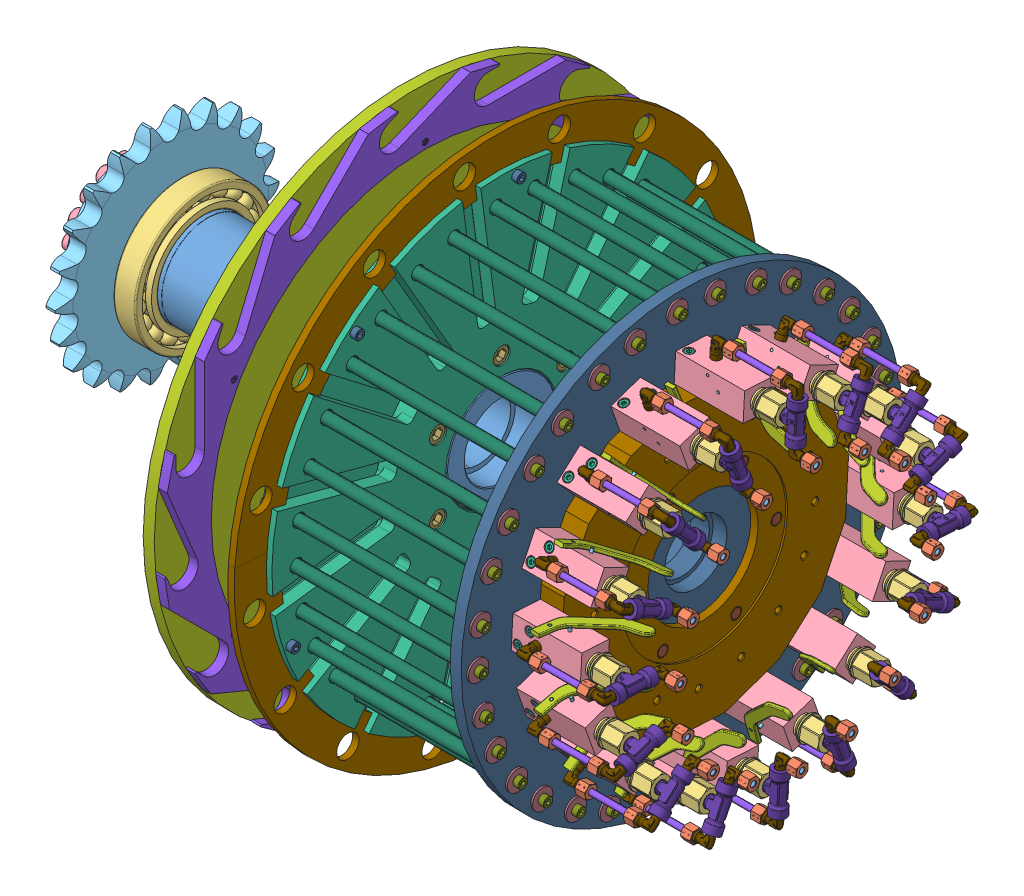
SolidWorks assembly assieme parte rotante, configuration Default. Lengths in mm.
Overall size (749.63 778.63 778.63).
555 component instances, 28 part files, 75 mates.
Components (placement in the parent):
- albero rotazione piatti-1: albero rotazione piatti [Default] at (60.413 18.3637 415) size (415 200 200)
- seger 100mm-1: seger 100mm [KS 1336 E - 100] at (-146.4567 18.3637 415) x (0 0 -1) z (1 0 0) size (107.55 112.98 3)
- SKF - 6020 - 20,DE,NC,20_68-1: SKF - 6020 - 20,DE,NC,20_68 [SKF - 6020 - 20,DE,NC,20_68] at (-131.4567 18.3637 415) x (1 0 0) z (0 -0.434476 -0.900684) size (24 150 150)
- calettatore d95-1: calettatore d95 [Default] at (-184.9572 18.3637 415) size (39.5 135 135)
- pulegia z =50-1: pulegia z =50 [Chain wheel ISO - 22Z 20A-1 --22SB150H40L95.0N] at (-173.9167 18.3637 415) size (40 241.57 243.73)
- Disco supporto montaggio e Colonne-1: Disco supporto montaggio e Colonne [Default] at (204.0433 18.3637 415) x (0 -0.866025 -0.5) z (1 0 0) size (499.6 499.6 29)
- SKF - 6020 - 20,DE,NC,20_68-2: SKF - 6020 - 20,DE,NC,20_68 [SKF - 6020 - 20,DE,NC,20_68] at (62.0433 18.3637 415) x (1 0 0) z (0 -0.432628 -0.901573) size (24 150 150)
- piatto rotante porta tappi-1: piatto rotante porta tappi [Default] at (99.0433 18.3637 415) x (0 0 -1) z (1 0 0) size (570 570 20.57)
- disco trasportatore tappi 31-1: disco trasportatore tappi 31 [Default] at (111.0433 18.3637 415) x (0 0.5 -0.866025) z (1 0 0) size (570 570 10.42)
- Distributore Rotante-1: Distributore Rotante [Default] at (425.0433 18.3637 415) x (0 -0.055301 -0.99847) z (1 0 0) size (310 310 25.54)
- disco trascinato porta distributore vuoto-1: disco trascinato porta distributore vuoto [Default] at (400.0433 18.3637 415) x (0 0.055301 0.99847) z (-1 0 0) size (480 480 50)
- m12 35mm-1: m12 35mm [ISO 4762 M12 x 35 - 35N] at (376.0433 -53.0243 378.8925) x (1 0 0) z (0 -0.5 0.866025) size (47 18 18)
- m12 90mm-3: m12 90mm [ISO 4762 M12 x 90 - 90N] at (203.0433 -21.6363 345.718) x (-1 0 0) z (0 -0.5 0.866025) size (102 18 18)
- rondella m6 22mm-1: rondella m6 22mm [Washer ISO 7094 - 6] at (99.0433 -101.6363 207.1539) x (1 0 0) z (0 -1 0) size (2 22 22)
- M6 20mm-1: M6 20mm [ISO 4762 M6 x 20 - 20N] at (91.0433 -101.6363 207.1539) x (1 0 0) z (0 0.5 0.866025) size (26 10 10)
- m12 35mm-2: m12 35mm [ISO 4762 M12 x 35 - 35N] at (376.0433 13.9397 335.1224) x (1 0 0) z (0 -1 0) size (47 18 18)
- m12 35mm-3: m12 35mm [ISO 4762 M12 x 35 - 35N] at (376.0433 85.3277 371.2299) x (1 0 0) z (0 -0.5 -0.866025) size (47 18 18)
- m12 35mm-4: m12 35mm [ISO 4762 M12 x 35 - 35N] at (376.0433 89.7517 451.1075) x (1 0 0) z (0 0.5 -0.866025) size (47 18 18)
- m12 35mm-5: m12 35mm [ISO 4762 M12 x 35 - 35N] at (376.0433 22.7877 494.8776) x (1 0 0) z (0 1 0) size (47 18 18)
- m12 35mm-6: m12 35mm [ISO 4762 M12 x 35 - 35N] at (376.0433 -48.6003 458.7701) x (1 0 0) z (0 0.5 0.866025) size (47 18 18)
- rondella m6 22mm-2: rondella m6 22mm [Washer ISO 7094 - 6] at (99.0433 138.3637 207.1539) x (1 0 0) z (0 -0.5 -0.866025) size (2 22 22)
- rondella m6 22mm-3: rondella m6 22mm [Washer ISO 7094 - 6] at (99.0433 258.3637 415) x (1 0 0) z (0 0.5 -0.866025) size (2 22 22)
- rondella m6 22mm-4: rondella m6 22mm [Washer ISO 7094 - 6] at (99.0433 138.3637 622.8461) x (1 0 0) z (0 1 0) size (2 22 22)
- rondella m6 22mm-5: rondella m6 22mm [Washer ISO 7094 - 6] at (99.0433 -101.6363 622.8461) x (1 0 0) z (0 0.5 0.866025) size (2 22 22)
- rondella m6 22mm-6: rondella m6 22mm [Washer ISO 7094 - 6] at (99.0433 -221.6363 415) x (1 0 0) z (0 -0.5 0.866025) size (2 22 22)
- M6 20mm-2: M6 20mm [ISO 4762 M6 x 20 - 20N] at (91.0433 138.3637 207.1539) x (1 0 0) z (0 -0.5 0.866025) size (26 10 10)
- M6 20mm-3: M6 20mm [ISO 4762 M6 x 20 - 20N] at (91.0433 258.3637 415) x (1 0 0) z (0 -1 0) size (26 10 10)
- M6 20mm-4: M6 20mm [ISO 4762 M6 x 20 - 20N] at (91.0433 138.3637 622.8461) x (1 0 0) z (0 -0.5 -0.866025) size (26 10 10)
- M6 20mm-5: M6 20mm [ISO 4762 M6 x 20 - 20N] at (91.0433 -101.6363 622.8461) x (1 0 0) z (0 0.5 -0.866025) size (26 10 10)
- M6 20mm-6: M6 20mm [ISO 4762 M6 x 20 - 20N] at (91.0433 -221.6363 415) x (1 0 0) z (0 1 0) size (26 10 10)
- m12 90mm-4: m12 90mm [ISO 4762 M12 x 90 - 90N] at (203.0433 58.3637 345.718) x (-1 0 0) z (0 -1 0) size (102 18 18)
- m12 90mm-5: m12 90mm [ISO 4762 M12 x 90 - 90N] at (203.0433 98.3637 415) x (-1 0 0) z (0 -0.5 -0.866025) size (102 18 18)
- m12 90mm-6: m12 90mm [ISO 4762 M12 x 90 - 90N] at (203.0433 58.3637 484.282) x (-1 0 0) z (0 0.5 -0.866025) size (102 18 18)
- m12 90mm-7: m12 90mm [ISO 4762 M12 x 90 - 90N] at (203.0433 -21.6363 484.282) x (-1 0 0) z (0 1 0) size (102 18 18)
- m12 90mm-8: m12 90mm [ISO 4762 M12 x 90 - 90N] at (203.0433 -61.6363 415) x (-1 0 0) z (0 0.5 0.866025) size (102 18 18)
- asta scorrimento carello-1: asta scorrimento carello [Default] at (287.5433 70.1437 197.9013) x (0 0 -1) z (1 0 0) size (12 12 225)
- rondella m6 22mm-7: rondella m6 22mm [Washer ISO 7094 - 6] at (175.0433 70.1437 197.9013) x (1 0 0) z (0 -1 0) size (2 22 22)
- M6 16mm-1: M6 16mm [ISO 4762 M6 x 16 - 16N] at (167.0433 70.1437 197.9013) size (22 10 10)
- M6 16mm-2: M6 16mm [ISO 4762 M6 x 16 - 16N] at (408.0433 70.1437 197.9013) x (-1 0 0) z (0 0 -1) size (22 10 10)
- rondella m6 22mm-8: rondella m6 22mm [Washer ISO 7094 - 6] at (400.0433 70.1437 197.9013) x (-1 0 0) z (0 1 0) size (2 22 22)
- rondella m6 22mm-9: rondella m6 22mm [Washer ISO 7094 - 6] at (175.0433 24.5373 191.8971) x (1 0 0) z (0 -0.965926 -0.258819) size (2 22 22)
- M6 16mm-3: M6 16mm [ISO 4762 M6 x 16 - 16N] at (167.0433 24.5373 191.8971) x (1 0 0) z (0 0.258819 -0.965926) size (22 10 10)
- asta scorrimento carello-2: asta scorrimento carello [Default] at (287.5433 24.5373 191.8971) x (0 0.258819 -0.965926) z (-1 0 0) size (12 12 225)
- rondella m6 22mm-10: rondella m6 22mm [Washer ISO 7094 - 6] at (400.0433 24.5373 191.8971) x (-1 0 0) z (0 0.965926 0.258819) size (2 22 22)
- M6 16mm-4: M6 16mm [ISO 4762 M6 x 16 - 16N] at (408.0433 24.5373 191.8971) x (-1 0 0) z (0 -0.258819 0.965926) size (22 10 10)
- AssiemeValvola-1: AssiemeValvola [Default] at (515.3257 74.6348 254.5832) x (0 -0.331007 0.943628) z (0 0.943628 0.331007) size (90.26 138.63 38)
  - RaccordoT-1: RaccordoT [Default] at origin size (43 29.75 16.5)
  - Raccordo a L-1: Raccordo a L [Default] at (-30 0 0) x (0 -1 0) z (0 0 -1) size (28.34 25.51 14.01)
    - 1809_06_10_01-1: 1809_06_10_01 [Default] at origin size (22.49 23 10)
    - 1809_06_10_02-1: 1809_06_10_02 [Default] at origin size (6.5 8.5 8.5)
    - 1809_06_10_03-1: 1809_06_10_03 [Default] at origin size (11.02 15.01 14.01)
  - Raccordo a L-2: Raccordo a L [Default] at (30 0 0) x (0 1 0) z (0 0 -1) size (28.34 25.51 14.01)
    - 1809_06_10_01-1: 1809_06_10_01 [Default] at origin size (22.49 23 10)
    - 1809_06_10_02-1: 1809_06_10_02 [Default] at origin size (6.5 8.5 8.5)
    - 1809_06_10_03-1: 1809_06_10_03 [Default] at origin size (11.02 15.01 14.01)
  - TappoChiusura-1: TappoChiusura [Default] at (0 -32 0) x (0 -1 0) z (0 0 1) size (38.28 26.74 26.74)
  - CorpoValvola-1: CorpoValvola [Default] at (-15 -115.2824 0) size (30 75 34)
  - Raccordo a L-3: Raccordo a L [Default] at (-30 -88.2824 0) x (0 1 0) z (0 0 1) size (28.34 25.51 14.01)
    - 1809_06_10_01-1: 1809_06_10_01 [Default] at origin size (22.49 23 10)
    - 1809_06_10_02-1: 1809_06_10_02 [Default] at origin size (6.5 8.5 8.5)
    - 1809_06_10_03-1: 1809_06_10_03 [Default] at origin size (11.02 15.01 14.01)
  - Spina_3x38-1: Spina_3x38 [Default] at (0 -68.2824 -21) x (-1 0 0) z (0 0 1) size (3 3 38)
  - Spina_3x38-2: Spina_3x38 [Default] at (-10 -80.2824 -21) x (0.996193 0.087174 0) z (0 0 1) size (3 3 38)
  - M5 40mm-3: M5 40mm [ISO 4762 M5 x 40 - 40N] at (-14.6 -108.7824 9) size (45 8.5 8.5)
  - M5 40mm-2: M5 40mm [ISO 4762 M5 x 40 - 40N] at (-14.6 -96.7824 -9) size (45 8.5 8.5)
  - LevaValvola-1: LevaValvola [Default] at (-24.507 -86.571 -17) x (0.996193 0.087174 0) z (0 0 1) size (77.55 60.2 4)
  - Tubo-1: Tubo [Default] at (-30 -15.9665 0) x (1 0 0) z (0 -1 0) size (6 6 56.4)
- M6 16mm-5: M6 16mm [ISO 4762 M6 x 16 - 16N] at (167.0433 -16.8778 194.6116) x (1 0 0) z (0 0.382683 0.92388) size (22 10 10)
- M6 16mm-6: M6 16mm [ISO 4762 M6 x 16 - 16N] at (167.0433 -98.5342 224.874) x (1 0 0) z (0 0.707107 0.707107) size (22 10 10)
- M6 16mm-7: M6 16mm [ISO 4762 M6 x 16 - 16N] at (167.0433 -162.3939 284.0814) x (1 0 0) z (0 0.92388 0.382683) size (22 10 10)
- M6 16mm-8: M6 16mm [ISO 4762 M6 x 16 - 16N] at (167.0433 -198.735 363.22) x (1 0 0) z (0 1 0) size (22 10 10)
- M6 16mm-9: M6 16mm [ISO 4762 M6 x 16 - 16N] at (167.0433 -202.0247 450.2415) x (1 0 0) z (0 0.92388 -0.382683) size (22 10 10)
- M6 16mm-10: M6 16mm [ISO 4762 M6 x 16 - 16N] at (167.0433 -171.7623 531.8979) x (1 0 0) z (0 0.707107 -0.707107) size (22 10 10)
- M6 16mm-11: M6 16mm [ISO 4762 M6 x 16 - 16N] at (167.0433 -112.5549 595.7576) x (1 0 0) z (0 0.382683 -0.92388) size (22 10 10)
- M6 16mm-12: M6 16mm [ISO 4762 M6 x 16 - 16N] at (167.0433 -33.4163 632.0987) x (1 0 0) z (0 0 -1) size (22 10 10)
- M6 16mm-13: M6 16mm [ISO 4762 M6 x 16 - 16N] at (167.0433 53.6052 635.3884) x (1 0 0) z (0 -0.382683 -0.92388) size (22 10 10)
- M6 16mm-14: M6 16mm [ISO 4762 M6 x 16 - 16N] at (167.0433 135.2616 605.126) x (1 0 0) z (0 -0.707107 -0.707107) size (22 10 10)
- M6 16mm-15: M6 16mm [ISO 4762 M6 x 16 - 16N] at (167.0433 199.1213 545.9186) x (1 0 0) z (0 -0.92388 -0.382683) size (22 10 10)
- M6 16mm-16: M6 16mm [ISO 4762 M6 x 16 - 16N] at (167.0433 235.4624 466.78) x (1 0 0) z (0 -1 0) size (22 10 10)
- M6 16mm-17: M6 16mm [ISO 4762 M6 x 16 - 16N] at (167.0433 238.7521 379.7585) x (1 0 0) z (0 -0.92388 0.382683) size (22 10 10)
- M6 16mm-18: M6 16mm [ISO 4762 M6 x 16 - 16N] at (167.0433 208.4897 298.1021) x (1 0 0) z (0 -0.707107 0.707107) size (22 10 10)
- M6 16mm-19: M6 16mm [ISO 4762 M6 x 16 - 16N] at (167.0433 149.2823 234.2424) x (1 0 0) z (0 -0.382683 0.92388) size (22 10 10)
- rondella m6 22mm-11: rondella m6 22mm [Washer ISO 7094 - 6] at (175.0433 -16.8778 194.6116) x (1 0 0) z (0 -0.92388 0.382683) size (2 22 22)
- rondella m6 22mm-12: rondella m6 22mm [Washer ISO 7094 - 6] at (175.0433 -98.5342 224.874) x (1 0 0) z (0 -0.707107 0.707107) size (2 22 22)
- rondella m6 22mm-13: rondella m6 22mm [Washer ISO 7094 - 6] at (175.0433 -162.3939 284.0814) x (1 0 0) z (0 -0.382683 0.92388) size (2 22 22)
- rondella m6 22mm-14: rondella m6 22mm [Washer ISO 7094 - 6] at (175.0433 -198.735 363.22) size (2 22 22)
- rondella m6 22mm-15: rondella m6 22mm [Washer ISO 7094 - 6] at (175.0433 -202.0247 450.2415) x (1 0 0) z (0 0.382683 0.92388) size (2 22 22)
- rondella m6 22mm-16: rondella m6 22mm [Washer ISO 7094 - 6] at (175.0433 -171.7623 531.8979) x (1 0 0) z (0 0.707107 0.707107) size (2 22 22)
- rondella m6 22mm-17: rondella m6 22mm [Washer ISO 7094 - 6] at (175.0433 -112.5549 595.7576) x (1 0 0) z (0 0.92388 0.382683) size (2 22 22)
- rondella m6 22mm-18: rondella m6 22mm [Washer ISO 7094 - 6] at (175.0433 -33.4163 632.0987) x (1 0 0) z (0 1 0) size (2 22 22)
- rondella m6 22mm-19: rondella m6 22mm [Washer ISO 7094 - 6] at (175.0433 53.6052 635.3884) x (1 0 0) z (0 0.92388 -0.382683) size (2 22 22)
- rondella m6 22mm-20: rondella m6 22mm [Washer ISO 7094 - 6] at (175.0433 135.2616 605.126) x (1 0 0) z (0 0.707107 -0.707107) size (2 22 22)
- rondella m6 22mm-21: rondella m6 22mm [Washer ISO 7094 - 6] at (175.0433 199.1213 545.9186) x (1 0 0) z (0 0.382683 -0.92388) size (2 22 22)
- rondella m6 22mm-22: rondella m6 22mm [Washer ISO 7094 - 6] at (175.0433 235.4624 466.78) x (1 0 0) z (0 0 -1) size (2 22 22)
- rondella m6 22mm-23: rondella m6 22mm [Washer ISO 7094 - 6] at (175.0433 238.7521 379.7585) x (1 0 0) z (0 -0.382683 -0.92388) size (2 22 22)
- rondella m6 22mm-24: rondella m6 22mm [Washer ISO 7094 - 6] at (175.0433 208.4897 298.1021) x (1 0 0) z (0 -0.707107 -0.707107) size (2 22 22)
- rondella m6 22mm-25: rondella m6 22mm [Washer ISO 7094 - 6] at (175.0433 149.2823 234.2424) x (1 0 0) z (0 -0.92388 -0.382683) size (2 22 22)
- asta scorrimento carello-3: asta scorrimento carello [Default] at (287.5433 -16.8778 194.6116) x (0 -0.382683 -0.92388) z (1 0 0) size (12 12 225)
- asta scorrimento carello-4: asta scorrimento carello [Default] at (287.5433 -98.5342 224.874) x (0 -0.707107 -0.707107) z (1 0 0) size (12 12 225)
- asta scorrimento carello-5: asta scorrimento carello [Default] at (287.5433 -162.3939 284.0814) x (0 -0.92388 -0.382683) z (1 0 0) size (12 12 225)
- asta scorrimento carello-6: asta scorrimento carello [Default] at (287.5433 -198.735 363.22) x (0 -1 0) z (1 0 0) size (12 12 225)
- asta scorrimento carello-7: asta scorrimento carello [Default] at (287.5433 -202.0247 450.2415) x (0 -0.92388 0.382683) z (1 0 0) size (12 12 225)
- asta scorrimento carello-8: asta scorrimento carello [Default] at (287.5433 -171.7623 531.8979) x (0 -0.707107 0.707107) z (1 0 0) size (12 12 225)
- asta scorrimento carello-9: asta scorrimento carello [Default] at (287.5433 -112.5549 595.7576) x (0 -0.382683 0.92388) z (1 0 0) size (12 12 225)
- asta scorrimento carello-10: asta scorrimento carello [Default] at (287.5433 -33.4163 632.0987) x (0 0 1) z (1 0 0) size (12 12 225)
- asta scorrimento carello-11: asta scorrimento carello [Default] at (287.5433 53.6052 635.3884) x (0 0.382683 0.92388) z (1 0 0) size (12 12 225)
- asta scorrimento carello-12: asta scorrimento carello [Default] at (287.5433 135.2616 605.126) x (0 0.707107 0.707107) z (1 0 0) size (12 12 225)
- asta scorrimento carello-13: asta scorrimento carello [Default] at (287.5433 199.1213 545.9186) x (0 0.92388 0.382683) z (1 0 0) size (12 12 225)
- asta scorrimento carello-14: asta scorrimento carello [Default] at (287.5433 235.4624 466.78) x (0 1 0) z (1 0 0) size (12 12 225)
- asta scorrimento carello-15: asta scorrimento carello [Default] at (287.5433 238.7521 379.7585) x (0 0.92388 -0.382683) z (1 0 0) size (12 12 225)
- asta scorrimento carello-16: asta scorrimento carello [Default] at (287.5433 208.4897 298.1021) x (0 0.707107 -0.707107) z (1 0 0) size (12 12 225)
- asta scorrimento carello-17: asta scorrimento carello [Default] at (287.5433 149.2823 234.2424) x (0 0.382683 -0.92388) z (1 0 0) size (12 12 225)
- M6 16mm-20: M6 16mm [ISO 4762 M6 x 16 - 16N] at (408.0433 -16.8778 194.6116) x (-1 0 0) z (0 -0.382683 -0.92388) size (22 10 10)
- M6 16mm-21: M6 16mm [ISO 4762 M6 x 16 - 16N] at (408.0433 -98.5342 224.874) x (-1 0 0) z (0 -0.707107 -0.707107) size (22 10 10)
- M6 16mm-22: M6 16mm [ISO 4762 M6 x 16 - 16N] at (408.0433 -162.3939 284.0814) x (-1 0 0) z (0 -0.92388 -0.382683) size (22 10 10)
- M6 16mm-23: M6 16mm [ISO 4762 M6 x 16 - 16N] at (408.0433 -198.735 363.22) x (-1 0 0) z (0 -1 0) size (22 10 10)
- M6 16mm-24: M6 16mm [ISO 4762 M6 x 16 - 16N] at (408.0433 -202.0247 450.2415) x (-1 0 0) z (0 -0.92388 0.382683) size (22 10 10)
- M6 16mm-25: M6 16mm [ISO 4762 M6 x 16 - 16N] at (408.0433 -171.7623 531.8979) x (-1 0 0) z (0 -0.707107 0.707107) size (22 10 10)
- M6 16mm-26: M6 16mm [ISO 4762 M6 x 16 - 16N] at (408.0433 -112.5549 595.7576) x (-1 0 0) z (0 -0.382683 0.92388) size (22 10 10)
- M6 16mm-27: M6 16mm [ISO 4762 M6 x 16 - 16N] at (408.0433 -33.4163 632.0987) x (-1 0 0) z (0 0 1) size (22 10 10)
- M6 16mm-28: M6 16mm [ISO 4762 M6 x 16 - 16N] at (408.0433 53.6052 635.3884) x (-1 0 0) z (0 0.382683 0.92388) size (22 10 10)
- M6 16mm-29: M6 16mm [ISO 4762 M6 x 16 - 16N] at (408.0433 135.2616 605.126) x (-1 0 0) z (0 0.707107 0.707107) size (22 10 10)
- M6 16mm-30: M6 16mm [ISO 4762 M6 x 16 - 16N] at (408.0433 199.1213 545.9186) x (-1 0 0) z (0 0.92388 0.382683) size (22 10 10)
- M6 16mm-31: M6 16mm [ISO 4762 M6 x 16 - 16N] at (408.0433 235.4624 466.78) x (-1 0 0) z (0 1 0) size (22 10 10)
- M6 16mm-32: M6 16mm [ISO 4762 M6 x 16 - 16N] at (408.0433 238.7521 379.7585) x (-1 0 0) z (0 0.92388 -0.382683) size (22 10 10)
- M6 16mm-33: M6 16mm [ISO 4762 M6 x 16 - 16N] at (408.0433 208.4897 298.1021) x (-1 0 0) z (0 0.707107 -0.707107) size (22 10 10)
- M6 16mm-34: M6 16mm [ISO 4762 M6 x 16 - 16N] at (408.0433 149.2823 234.2424) x (-1 0 0) z (0 0.382683 -0.92388) size (22 10 10)
- rondella m6 22mm-26: rondella m6 22mm [Washer ISO 7094 - 6] at (400.0433 -16.8778 194.6116) x (-1 0 0) z (0 0.92388 -0.382683) size (2 22 22)
- rondella m6 22mm-27: rondella m6 22mm [Washer ISO 7094 - 6] at (400.0433 -98.5342 224.874) x (-1 0 0) z (0 0.707107 -0.707107) size (2 22 22)
- rondella m6 22mm-28: rondella m6 22mm [Washer ISO 7094 - 6] at (400.0433 -162.3939 284.0814) x (-1 0 0) z (0 0.382683 -0.92388) size (2 22 22)
- rondella m6 22mm-29: rondella m6 22mm [Washer ISO 7094 - 6] at (400.0433 -198.735 363.22) x (-1 0 0) z (0 0 -1) size (2 22 22)
- rondella m6 22mm-30: rondella m6 22mm [Washer ISO 7094 - 6] at (400.0433 -202.0247 450.2415) x (-1 0 0) z (0 -0.382683 -0.92388) size (2 22 22)
- rondella m6 22mm-31: rondella m6 22mm [Washer ISO 7094 - 6] at (400.0433 -171.7623 531.8979) x (-1 0 0) z (0 -0.707107 -0.707107) size (2 22 22)
- rondella m6 22mm-32: rondella m6 22mm [Washer ISO 7094 - 6] at (400.0433 -112.5549 595.7576) x (-1 0 0) z (0 -0.92388 -0.382683) size (2 22 22)
- rondella m6 22mm-33: rondella m6 22mm [Washer ISO 7094 - 6] at (400.0433 -33.4163 632.0987) x (-1 0 0) z (0 -1 0) size (2 22 22)
- rondella m6 22mm-34: rondella m6 22mm [Washer ISO 7094 - 6] at (400.0433 53.6052 635.3884) x (-1 0 0) z (0 -0.92388 0.382683) size (2 22 22)
- rondella m6 22mm-35: rondella m6 22mm [Washer ISO 7094 - 6] at (400.0433 135.2616 605.126) x (-1 0 0) z (0 -0.707107 0.707107) size (2 22 22)
- rondella m6 22mm-36: rondella m6 22mm [Washer ISO 7094 - 6] at (400.0433 199.1213 545.9186) x (-1 0 0) z (0 -0.382683 0.92388) size (2 22 22)
- rondella m6 22mm-37: rondella m6 22mm [Washer ISO 7094 - 6] at (400.0433 235.4624 466.78) x (-1 0 0) z (0 0 1) size (2 22 22)
- rondella m6 22mm-38: rondella m6 22mm [Washer ISO 7094 - 6] at (400.0433 238.7521 379.7585) x (-1 0 0) z (0 0.382683 0.92388) size (2 22 22)
- rondella m6 22mm-39: rondella m6 22mm [Washer ISO 7094 - 6] at (400.0433 208.4897 298.1021) x (-1 0 0) z (0 0.707107 0.707107) size (2 22 22)
- rondella m6 22mm-40: rondella m6 22mm [Washer ISO 7094 - 6] at (400.0433 149.2823 234.2424) x (-1 0 0) z (0 0.92388 0.382683) size (2 22 22)
- rondella m6 22mm-41: rondella m6 22mm [Washer ISO 7094 - 6] at (175.0433 -61.3104 206.5173) x (1 0 0) z (0 -0.991445 0.130526) size (2 22 22)
- rondella m6 22mm-42: rondella m6 22mm [Washer ISO 7094 - 6] at (175.0433 -135.0285 252.8771) x (1 0 0) z (0 -0.866025 0.5) size (2 22 22)
- rondella m6 22mm-43: rondella m6 22mm [Washer ISO 7094 - 6] at (175.0433 -185.3939 323.9186) x (1 0 0) z (0 -0.608761 0.793353) size (2 22 22)
- rondella m6 22mm-44: rondella m6 22mm [Washer ISO 7094 - 6] at (175.0433 -204.7392 408.8264) x (1 0 0) z (0 -0.258819 0.965926) size (2 22 22)
- rondella m6 22mm-45: rondella m6 22mm [Washer ISO 7094 - 6] at (175.0433 -190.119 494.6741) x (1 0 0) z (0 0.130526 0.991445) size (2 22 22)
- rondella m6 22mm-46: rondella m6 22mm [Washer ISO 7094 - 6] at (175.0433 -143.7592 568.3922) x (1 0 0) z (0 0.5 0.866025) size (2 22 22)
- rondella m6 22mm-47: rondella m6 22mm [Washer ISO 7094 - 6] at (175.0433 -72.7177 618.7576) x (1 0 0) z (0 0.793353 0.608761) size (2 22 22)
- rondella m6 22mm-48: rondella m6 22mm [Washer ISO 7094 - 6] at (175.0433 12.1901 638.1029) x (1 0 0) z (0 0.965926 0.258819) size (2 22 22)
- rondella m6 22mm-49: rondella m6 22mm [Washer ISO 7094 - 6] at (175.0433 98.0378 623.4827) x (1 0 0) z (0 0.991445 -0.130526) size (2 22 22)
- rondella m6 22mm-50: rondella m6 22mm [Washer ISO 7094 - 6] at (175.0433 171.7559 577.1229) x (1 0 0) z (0 0.866025 -0.5) size (2 22 22)
- rondella m6 22mm-51: rondella m6 22mm [Washer ISO 7094 - 6] at (175.0433 222.1213 506.0814) x (1 0 0) z (0 0.608761 -0.793353) size (2 22 22)
- rondella m6 22mm-52: rondella m6 22mm [Washer ISO 7094 - 6] at (175.0433 241.4666 421.1736) x (1 0 0) z (0 0.258819 -0.965926) size (2 22 22)
- rondella m6 22mm-53: rondella m6 22mm [Washer ISO 7094 - 6] at (175.0433 226.8464 335.3259) x (1 0 0) z (0 -0.130526 -0.991445) size (2 22 22)
- rondella m6 22mm-54: rondella m6 22mm [Washer ISO 7094 - 6] at (175.0433 180.4866 261.6078) x (1 0 0) z (0 -0.5 -0.866025) size (2 22 22)
- rondella m6 22mm-55: rondella m6 22mm [Washer ISO 7094 - 6] at (175.0433 109.4451 211.2424) x (1 0 0) z (0 -0.793353 -0.608761) size (2 22 22)
- M6 16mm-35: M6 16mm [ISO 4762 M6 x 16 - 16N] at (167.0433 -61.3104 206.5173) x (1 0 0) z (0 -0.130526 -0.991445) size (22 10 10)
- M6 16mm-36: M6 16mm [ISO 4762 M6 x 16 - 16N] at (167.0433 -135.0285 252.8771) x (1 0 0) z (0 -0.5 -0.866025) size (22 10 10)
- M6 16mm-37: M6 16mm [ISO 4762 M6 x 16 - 16N] at (167.0433 -185.3939 323.9186) x (1 0 0) z (0 -0.793353 -0.608761) size (22 10 10)
- M6 16mm-38: M6 16mm [ISO 4762 M6 x 16 - 16N] at (167.0433 -204.7392 408.8264) x (1 0 0) z (0 -0.965926 -0.258819) size (22 10 10)
- M6 16mm-39: M6 16mm [ISO 4762 M6 x 16 - 16N] at (167.0433 -190.119 494.6741) x (1 0 0) z (0 -0.991445 0.130526) size (22 10 10)
- M6 16mm-40: M6 16mm [ISO 4762 M6 x 16 - 16N] at (167.0433 -143.7592 568.3922) x (1 0 0) z (0 -0.866025 0.5) size (22 10 10)
- M6 16mm-41: M6 16mm [ISO 4762 M6 x 16 - 16N] at (167.0433 -72.7177 618.7576) x (1 0 0) z (0 -0.608761 0.793353) size (22 10 10)
- M6 16mm-42: M6 16mm [ISO 4762 M6 x 16 - 16N] at (167.0433 12.1901 638.1029) x (1 0 0) z (0 -0.258819 0.965926) size (22 10 10)
- M6 16mm-43: M6 16mm [ISO 4762 M6 x 16 - 16N] at (167.0433 98.0378 623.4827) x (1 0 0) z (0 0.130526 0.991445) size (22 10 10)
- M6 16mm-44: M6 16mm [ISO 4762 M6 x 16 - 16N] at (167.0433 171.7559 577.1229) x (1 0 0) z (0 0.5 0.866025) size (22 10 10)
- M6 16mm-45: M6 16mm [ISO 4762 M6 x 16 - 16N] at (167.0433 222.1213 506.0814) x (1 0 0) z (0 0.793353 0.608761) size (22 10 10)
- M6 16mm-46: M6 16mm [ISO 4762 M6 x 16 - 16N] at (167.0433 241.4666 421.1736) x (1 0 0) z (0 0.965926 0.258819) size (22 10 10)
- M6 16mm-47: M6 16mm [ISO 4762 M6 x 16 - 16N] at (167.0433 226.8464 335.3259) x (1 0 0) z (0 0.991445 -0.130526) size (22 10 10)
- M6 16mm-48: M6 16mm [ISO 4762 M6 x 16 - 16N] at (167.0433 180.4866 261.6078) x (1 0 0) z (0 0.866025 -0.5) size (22 10 10)
- M6 16mm-49: M6 16mm [ISO 4762 M6 x 16 - 16N] at (167.0433 109.4451 211.2424) x (1 0 0) z (0 0.608761 -0.793353) size (22 10 10)
- asta scorrimento carello-18: asta scorrimento carello [Default] at (287.5433 -61.3104 206.5173) x (0 -0.130526 -0.991445) z (-1 0 0) size (12 12 225)
- asta scorrimento carello-19: asta scorrimento carello [Default] at (287.5433 -135.0285 252.8771) x (0 -0.5 -0.866025) z (-1 0 0) size (12 12 225)
- asta scorrimento carello-20: asta scorrimento carello [Default] at (287.5433 -185.3939 323.9186) x (0 -0.793353 -0.608761) z (-1 0 0) size (12 12 225)
- asta scorrimento carello-21: asta scorrimento carello [Default] at (287.5433 -204.7392 408.8264) x (0 -0.965926 -0.258819) z (-1 0 0) size (12 12 225)
- asta scorrimento carello-22: asta scorrimento carello [Default] at (287.5433 -190.119 494.6741) x (0 -0.991445 0.130526) z (-1 0 0) size (12 12 225)
- asta scorrimento carello-23: asta scorrimento carello [Default] at (287.5433 -143.7592 568.3922) x (0 -0.866025 0.5) z (-1 0 0) size (12 12 225)
- asta scorrimento carello-24: asta scorrimento carello [Default] at (287.5433 -72.7177 618.7576) x (0 -0.608761 0.793353) z (-1 0 0) size (12 12 225)
- asta scorrimento carello-25: asta scorrimento carello [Default] at (287.5433 12.1901 638.1029) x (0 -0.258819 0.965926) z (-1 0 0) size (12 12 225)
- asta scorrimento carello-26: asta scorrimento carello [Default] at (287.5433 98.0378 623.4827) x (0 0.130526 0.991445) z (-1 0 0) size (12 12 225)
- asta scorrimento carello-27: asta scorrimento carello [Default] at (287.5433 171.7559 577.1229) x (0 0.5 0.866025) z (-1 0 0) size (12 12 225)
- asta scorrimento carello-28: asta scorrimento carello [Default] at (287.5433 222.1213 506.0814) x (0 0.793353 0.608761) z (-1 0 0) size (12 12 225)
- asta scorrimento carello-29: asta scorrimento carello [Default] at (287.5433 241.4666 421.1736) x (0 0.965926 0.258819) z (-1 0 0) size (12 12 225)
- asta scorrimento carello-30: asta scorrimento carello [Default] at (287.5433 226.8464 335.3259) x (0 0.991445 -0.130526) z (-1 0 0) size (12 12 225)
- asta scorrimento carello-31: asta scorrimento carello [Default] at (287.5433 180.4866 261.6078) x (0 0.866025 -0.5) z (-1 0 0) size (12 12 225)
- asta scorrimento carello-32: asta scorrimento carello [Default] at (287.5433 109.4451 211.2424) x (0 0.608761 -0.793353) z (-1 0 0) size (12 12 225)
- rondella m6 22mm-56: rondella m6 22mm [Washer ISO 7094 - 6] at (400.0433 -61.3104 206.5173) x (-1 0 0) z (0 0.991445 -0.130526) size (2 22 22)
- rondella m6 22mm-57: rondella m6 22mm [Washer ISO 7094 - 6] at (400.0433 -135.0285 252.8771) x (-1 0 0) z (0 0.866025 -0.5) size (2 22 22)
- rondella m6 22mm-58: rondella m6 22mm [Washer ISO 7094 - 6] at (400.0433 -185.3939 323.9186) x (-1 0 0) z (0 0.608761 -0.793353) size (2 22 22)
- rondella m6 22mm-59: rondella m6 22mm [Washer ISO 7094 - 6] at (400.0433 -204.7392 408.8264) x (-1 0 0) z (0 0.258819 -0.965926) size (2 22 22)
- rondella m6 22mm-60: rondella m6 22mm [Washer ISO 7094 - 6] at (400.0433 -190.119 494.6741) x (-1 0 0) z (0 -0.130526 -0.991445) size (2 22 22)
- rondella m6 22mm-61: rondella m6 22mm [Washer ISO 7094 - 6] at (400.0433 -143.7592 568.3922) x (-1 0 0) z (0 -0.5 -0.866025) size (2 22 22)
- rondella m6 22mm-62: rondella m6 22mm [Washer ISO 7094 - 6] at (400.0433 -72.7177 618.7576) x (-1 0 0) z (0 -0.793353 -0.608761) size (2 22 22)
- rondella m6 22mm-63: rondella m6 22mm [Washer ISO 7094 - 6] at (400.0433 12.1901 638.1029) x (-1 0 0) z (0 -0.965926 -0.258819) size (2 22 22)
- rondella m6 22mm-64: rondella m6 22mm [Washer ISO 7094 - 6] at (400.0433 98.0378 623.4827) x (-1 0 0) z (0 -0.991445 0.130526) size (2 22 22)
- rondella m6 22mm-65: rondella m6 22mm [Washer ISO 7094 - 6] at (400.0433 171.7559 577.1229) x (-1 0 0) z (0 -0.866025 0.5) size (2 22 22)
- rondella m6 22mm-66: rondella m6 22mm [Washer ISO 7094 - 6] at (400.0433 222.1213 506.0814) x (-1 0 0) z (0 -0.608761 0.793353) size (2 22 22)
- rondella m6 22mm-67: rondella m6 22mm [Washer ISO 7094 - 6] at (400.0433 241.4666 421.1736) x (-1 0 0) z (0 -0.258819 0.965926) size (2 22 22)
- rondella m6 22mm-68: rondella m6 22mm [Washer ISO 7094 - 6] at (400.0433 226.8464 335.3259) x (-1 0 0) z (0 0.130526 0.991445) size (2 22 22)
- rondella m6 22mm-69: rondella m6 22mm [Washer ISO 7094 - 6] at (400.0433 180.4866 261.6078) x (-1 0 0) z (0 0.5 0.866025) size (2 22 22)
- rondella m6 22mm-70: rondella m6 22mm [Washer ISO 7094 - 6] at (400.0433 109.4451 211.2424) x (-1 0 0) z (0 0.793353 0.608761) size (2 22 22)
- M6 16mm-50: M6 16mm [ISO 4762 M6 x 16 - 16N] at (408.0433 -61.3104 206.5173) x (-1 0 0) z (0 0.130526 0.991445) size (22 10 10)
- M6 16mm-51: M6 16mm [ISO 4762 M6 x 16 - 16N] at (408.0433 -135.0285 252.8771) x (-1 0 0) z (0 0.5 0.866025) size (22 10 10)
- M6 16mm-52: M6 16mm [ISO 4762 M6 x 16 - 16N] at (408.0433 -185.3939 323.9186) x (-1 0 0) z (0 0.793353 0.608761) size (22 10 10)
- M6 16mm-53: M6 16mm [ISO 4762 M6 x 16 - 16N] at (408.0433 -204.7392 408.8264) x (-1 0 0) z (0 0.965926 0.258819) size (22 10 10)
- M6 16mm-54: M6 16mm [ISO 4762 M6 x 16 - 16N] at (408.0433 -190.119 494.6741) x (-1 0 0) z (0 0.991445 -0.130526) size (22 10 10)
- M6 16mm-55: M6 16mm [ISO 4762 M6 x 16 - 16N] at (408.0433 -143.7592 568.3922) x (-1 0 0) z (0 0.866025 -0.5) size (22 10 10)
- M6 16mm-56: M6 16mm [ISO 4762 M6 x 16 - 16N] at (408.0433 -72.7177 618.7576) x (-1 0 0) z (0 0.608761 -0.793353) size (22 10 10)
- M6 16mm-57: M6 16mm [ISO 4762 M6 x 16 - 16N] at (408.0433 12.1901 638.1029) x (-1 0 0) z (0 0.258819 -0.965926) size (22 10 10)
- M6 16mm-58: M6 16mm [ISO 4762 M6 x 16 - 16N] at (408.0433 98.0378 623.4827) x (-1 0 0) z (0 -0.130526 -0.991445) size (22 10 10)
- M6 16mm-59: M6 16mm [ISO 4762 M6 x 16 - 16N] at (408.0433 171.7559 577.1229) x (-1 0 0) z (0 -0.5 -0.866025) size (22 10 10)
- M6 16mm-60: M6 16mm [ISO 4762 M6 x 16 - 16N] at (408.0433 222.1213 506.0814) x (-1 0 0) z (0 -0.793353 -0.608761) size (22 10 10)
- M6 16mm-61: M6 16mm [ISO 4762 M6 x 16 - 16N] at (408.0433 241.4666 421.1736) x (-1 0 0) z (0 -0.965926 -0.258819) size (22 10 10)
- M6 16mm-62: M6 16mm [ISO 4762 M6 x 16 - 16N] at (408.0433 226.8464 335.3259) x (-1 0 0) z (0 -0.991445 0.130526) size (22 10 10)
- M6 16mm-63: M6 16mm [ISO 4762 M6 x 16 - 16N] at (408.0433 180.4866 261.6078) x (-1 0 0) z (0 -0.866025 0.5) size (22 10 10)
- M6 16mm-64: M6 16mm [ISO 4762 M6 x 16 - 16N] at (408.0433 109.4451 211.2424) x (-1 0 0) z (0 -0.608761 0.793353) size (22 10 10)
- AssiemeValvola-2: AssiemeValvola [Default] at (515.3257 8.9626 245.2601) x (0 0.055301 0.99847) z (0 0.99847 -0.055301) size (90.26 138.63 38)
  - RaccordoT-1: RaccordoT [Default] at origin size (43 29.75 16.5)
  - Raccordo a L-1: Raccordo a L [Default] at (-30 0 0) x (0 -1 0) z (0 0 -1) size (28.34 25.51 14.01)
    - 1809_06_10_01-1: 1809_06_10_01 [Default] at origin size (22.49 23 10)
    - 1809_06_10_02-1: 1809_06_10_02 [Default] at origin size (6.5 8.5 8.5)
    - 1809_06_10_03-1: 1809_06_10_03 [Default] at origin size (11.02 15.01 14.01)
  - Raccordo a L-2: Raccordo a L [Default] at (30 0 0) x (0 1 0) z (0 0 -1) size (28.34 25.51 14.01)
    - 1809_06_10_01-1: 1809_06_10_01 [Default] at origin size (22.49 23 10)
    - 1809_06_10_02-1: 1809_06_10_02 [Default] at origin size (6.5 8.5 8.5)
    - 1809_06_10_03-1: 1809_06_10_03 [Default] at origin size (11.02 15.01 14.01)
  - TappoChiusura-1: TappoChiusura [Default] at (0 -32 0) x (0 -1 0) z (0 0 1) size (38.28 26.74 26.74)
  - CorpoValvola-1: CorpoValvola [Default] at (-15 -115.2824 0) size (30 75 34)
  - Raccordo a L-3: Raccordo a L [Default] at (-30 -88.2824 0) x (0 1 0) z (0 0 1) size (28.34 25.51 14.01)
    - 1809_06_10_01-1: 1809_06_10_01 [Default] at origin size (22.49 23 10)
    - 1809_06_10_02-1: 1809_06_10_02 [Default] at origin size (6.5 8.5 8.5)
    - 1809_06_10_03-1: 1809_06_10_03 [Default] at origin size (11.02 15.01 14.01)
  - Spina_3x38-1: Spina_3x38 [Default] at (0 -68.2824 -21) x (-1 0 0) z (0 0 1) size (3 3 38)
  - Spina_3x38-2: Spina_3x38 [Default] at (-10 -80.2824 -21) x (0.996193 0.087174 0) z (0 0 1) size (3 3 38)
  - M5 40mm-3: M5 40mm [ISO 4762 M5 x 40 - 40N] at (-14.6 -108.7824 9) size (45 8.5 8.5)
  - M5 40mm-2: M5 40mm [ISO 4762 M5 x 40 - 40N] at (-14.6 -96.7824 -9) size (45 8.5 8.5)
  - LevaValvola-1: LevaValvola [Default] at (-24.507 -86.571 -17) x (0.996193 0.087174 0) z (0 0 1) size (77.55 60.2 4)
  - Tubo-1: Tubo [Default] at (-30 -15.9665 0) x (1 0 0) z (0 -1 0) size (6 6 56.4)
- AssiemeValvola-3: AssiemeValvola [Default] at (515.3257 -55.2784 261.7785) x (0 0.433189 0.901303) z (0 0.901303 -0.433189) size (90.26 138.63 38)
  - RaccordoT-1: RaccordoT [Default] at origin size (43 29.75 16.5)
  - Raccordo a L-1: Raccordo a L [Default] at (-30 0 0) x (0 -1 0) z (0 0 -1) size (28.34 25.51 14.01)
    - 1809_06_10_01-1: 1809_06_10_01 [Default] at origin size (22.49 23 10)
    - 1809_06_10_02-1: 1809_06_10_02 [Default] at origin size (6.5 8.5 8.5)
    - 1809_06_10_03-1: 1809_06_10_03 [Default] at origin size (11.02 15.01 14.01)
  - Raccordo a L-2: Raccordo a L [Default] at (30 0 0) x (0 1 0) z (0 0 -1) size (28.34 25.51 14.01)
    - 1809_06_10_01-1: 1809_06_10_01 [Default] at origin size (22.49 23 10)
    - 1809_06_10_02-1: 1809_06_10_02 [Default] at origin size (6.5 8.5 8.5)
    - 1809_06_10_03-1: 1809_06_10_03 [Default] at origin size (11.02 15.01 14.01)
  - TappoChiusura-1: TappoChiusura [Default] at (0 -32 0) x (0 -1 0) z (0 0 1) size (38.28 26.74 26.74)
  - CorpoValvola-1: CorpoValvola [Default] at (-15 -115.2824 0) size (30 75 34)
  - Raccordo a L-3: Raccordo a L [Default] at (-30 -88.2824 0) x (0 1 0) z (0 0 1) size (28.34 25.51 14.01)
    - 1809_06_10_01-1: 1809_06_10_01 [Default] at origin size (22.49 23 10)
    - 1809_06_10_02-1: 1809_06_10_02 [Default] at origin size (6.5 8.5 8.5)
    - 1809_06_10_03-1: 1809_06_10_03 [Default] at origin size (11.02 15.01 14.01)
  - Spina_3x38-1: Spina_3x38 [Default] at (0 -68.2824 -21) x (-1 0 0) z (0 0 1) size (3 3 38)
  - Spina_3x38-2: Spina_3x38 [Default] at (-10 -80.2824 -21) x (0.996193 0.087174 0) z (0 0 1) size (3 3 38)
  - M5 40mm-3: M5 40mm [ISO 4762 M5 x 40 - 40N] at (-14.6 -108.7824 9) size (45 8.5 8.5)
  - M5 40mm-2: M5 40mm [ISO 4762 M5 x 40 - 40N] at (-14.6 -96.7824 -9) size (45 8.5 8.5)
  - LevaValvola-1: LevaValvola [Default] at (-24.507 -86.571 -17) x (0.996193 0.087174 0) z (0 0 1) size (77.55 60.2 4)
  - Tubo-1: Tubo [Default] at (-30 -15.9665 0) x (1 0 0) z (0 -1 0) size (6 6 56.4)
- AssiemeValvola-4: AssiemeValvola [Default] at (515.3257 -108.3081 301.6234) x (0 0.745128 0.666921) z (0 0.666921 -0.745128) size (90.26 138.63 38)
  - RaccordoT-1: RaccordoT [Default] at origin size (43 29.75 16.5)
  - Raccordo a L-1: Raccordo a L [Default] at (-30 0 0) x (0 -1 0) z (0 0 -1) size (28.34 25.51 14.01)
    - 1809_06_10_01-1: 1809_06_10_01 [Default] at origin size (22.49 23 10)
    - 1809_06_10_02-1: 1809_06_10_02 [Default] at origin size (6.5 8.5 8.5)
    - 1809_06_10_03-1: 1809_06_10_03 [Default] at origin size (11.02 15.01 14.01)
  - Raccordo a L-2: Raccordo a L [Default] at (30 0 0) x (0 1 0) z (0 0 -1) size (28.34 25.51 14.01)
    - 1809_06_10_01-1: 1809_06_10_01 [Default] at origin size (22.49 23 10)
    - 1809_06_10_02-1: 1809_06_10_02 [Default] at origin size (6.5 8.5 8.5)
    - 1809_06_10_03-1: 1809_06_10_03 [Default] at origin size (11.02 15.01 14.01)
  - TappoChiusura-1: TappoChiusura [Default] at (0 -32 0) x (0 -1 0) z (0 0 1) size (38.28 26.74 26.74)
  - CorpoValvola-1: CorpoValvola [Default] at (-15 -115.2824 0) size (30 75 34)
  - Raccordo a L-3: Raccordo a L [Default] at (-30 -88.2824 0) x (0 1 0) z (0 0 1) size (28.34 25.51 14.01)
    - 1809_06_10_01-1: 1809_06_10_01 [Default] at origin size (22.49 23 10)
    - 1809_06_10_02-1: 1809_06_10_02 [Default] at origin size (6.5 8.5 8.5)
    - 1809_06_10_03-1: 1809_06_10_03 [Default] at origin size (11.02 15.01 14.01)
  - Spina_3x38-1: Spina_3x38 [Default] at (0 -68.2824 -21) x (-1 0 0) z (0 0 1) size (3 3 38)
  - Spina_3x38-2: Spina_3x38 [Default] at (-10 -80.2824 -21) x (0.996193 0.087174 0) z (0 0 1) size (3 3 38)
  - M5 40mm-3: M5 40mm [ISO 4762 M5 x 40 - 40N] at (-14.6 -108.7824 9) size (45 8.5 8.5)
  - M5 40mm-2: M5 40mm [ISO 4762 M5 x 40 - 40N] at (-14.6 -96.7824 -9) size (45 8.5 8.5)
  - LevaValvola-1: LevaValvola [Default] at (-24.507 -86.571 -17) x (0.996193 0.087174 0) z (0 0 1) size (77.55 60.2 4)
  - Tubo-1: Tubo [Default] at (-30 -15.9665 0) x (1 0 0) z (0 -1 0) size (6 6 56.4)
- AssiemeValvola-5: AssiemeValvola [Default] at (515.3257 -142.0531 358.7289) x (0 0.943628 0.331007) z (0 0.331007 -0.943628) size (90.26 138.63 38)
  - RaccordoT-1: RaccordoT [Default] at origin size (43 29.75 16.5)
  - Raccordo a L-1: Raccordo a L [Default] at (-30 0 0) x (0 -1 0) z (0 0 -1) size (28.34 25.51 14.01)
    - 1809_06_10_01-1: 1809_06_10_01 [Default] at origin size (22.49 23 10)
    - 1809_06_10_02-1: 1809_06_10_02 [Default] at origin size (6.5 8.5 8.5)
    - 1809_06_10_03-1: 1809_06_10_03 [Default] at origin size (11.02 15.01 14.01)
  - Raccordo a L-2: Raccordo a L [Default] at (30 0 0) x (0 1 0) z (0 0 -1) size (28.34 25.51 14.01)
    - 1809_06_10_01-1: 1809_06_10_01 [Default] at origin size (22.49 23 10)
    - 1809_06_10_02-1: 1809_06_10_02 [Default] at origin size (6.5 8.5 8.5)
    - 1809_06_10_03-1: 1809_06_10_03 [Default] at origin size (11.02 15.01 14.01)
  - TappoChiusura-1: TappoChiusura [Default] at (0 -32 0) x (0 -1 0) z (0 0 1) size (38.28 26.74 26.74)
  - CorpoValvola-1: CorpoValvola [Default] at (-15 -115.2824 0) size (30 75 34)
  - Raccordo a L-3: Raccordo a L [Default] at (-30 -88.2824 0) x (0 1 0) z (0 0 1) size (28.34 25.51 14.01)
    - 1809_06_10_01-1: 1809_06_10_01 [Default] at origin size (22.49 23 10)
    - 1809_06_10_02-1: 1809_06_10_02 [Default] at origin size (6.5 8.5 8.5)
    - 1809_06_10_03-1: 1809_06_10_03 [Default] at origin size (11.02 15.01 14.01)
  - Spina_3x38-1: Spina_3x38 [Default] at (0 -68.2824 -21) x (-1 0 0) z (0 0 1) size (3 3 38)
  - Spina_3x38-2: Spina_3x38 [Default] at (-10 -80.2824 -21) x (0.996193 0.087174 0) z (0 0 1) size (3 3 38)
  - M5 40mm-3: M5 40mm [ISO 4762 M5 x 40 - 40N] at (-14.6 -108.7824 9) size (45 8.5 8.5)
  - M5 40mm-2: M5 40mm [ISO 4762 M5 x 40 - 40N] at (-14.6 -96.7824 -9) size (45 8.5 8.5)
  - LevaValvola-1: LevaValvola [Default] at (-24.507 -86.571 -17) x (0.996193 0.087174 0) z (0 0 1) size (77.55 60.2 4)
  - Tubo-1: Tubo [Default] at (-30 -15.9665 0) x (1 0 0) z (0 -1 0) size (6 6 56.4)
- AssiemeValvola-6: AssiemeValvola [Default] at (515.3257 -151.3762 424.4011) x (0 0.99847 -0.055301) z (0 -0.055301 -0.99847) size (90.26 138.63 38)
  - RaccordoT-1: RaccordoT [Default] at origin size (43 29.75 16.5)
  - Raccordo a L-1: Raccordo a L [Default] at (-30 0 0) x (0 -1 0) z (0 0 -1) size (28.34 25.51 14.01)
    - 1809_06_10_01-1: 1809_06_10_01 [Default] at origin size (22.49 23 10)
    - 1809_06_10_02-1: 1809_06_10_02 [Default] at origin size (6.5 8.5 8.5)
    - 1809_06_10_03-1: 1809_06_10_03 [Default] at origin size (11.02 15.01 14.01)
  - Raccordo a L-2: Raccordo a L [Default] at (30 0 0) x (0 1 0) z (0 0 -1) size (28.34 25.51 14.01)
    - 1809_06_10_01-1: 1809_06_10_01 [Default] at origin size (22.49 23 10)
    - 1809_06_10_02-1: 1809_06_10_02 [Default] at origin size (6.5 8.5 8.5)
    - 1809_06_10_03-1: 1809_06_10_03 [Default] at origin size (11.02 15.01 14.01)
  - TappoChiusura-1: TappoChiusura [Default] at (0 -32 0) x (0 -1 0) z (0 0 1) size (38.28 26.74 26.74)
  - CorpoValvola-1: CorpoValvola [Default] at (-15 -115.2824 0) size (30 75 34)
  - Raccordo a L-3: Raccordo a L [Default] at (-30 -88.2824 0) x (0 1 0) z (0 0 1) size (28.34 25.51 14.01)
    - 1809_06_10_01-1: 1809_06_10_01 [Default] at origin size (22.49 23 10)
    - 1809_06_10_02-1: 1809_06_10_02 [Default] at origin size (6.5 8.5 8.5)
    - 1809_06_10_03-1: 1809_06_10_03 [Default] at origin size (11.02 15.01 14.01)
  - Spina_3x38-1: Spina_3x38 [Default] at (0 -68.2824 -21) x (-1 0 0) z (0 0 1) size (3 3 38)
  - Spina_3x38-2: Spina_3x38 [Default] at (-10 -80.2824 -21) x (0.996193 0.087174 0) z (0 0 1) size (3 3 38)
  - M5 40mm-3: M5 40mm [ISO 4762 M5 x 40 - 40N] at (-14.6 -108.7824 9) size (45 8.5 8.5)
  - M5 40mm-2: M5 40mm [ISO 4762 M5 x 40 - 40N] at (-14.6 -96.7824 -9) size (45 8.5 8.5)
  - LevaValvola-1: LevaValvola [Default] at (-24.507 -86.571 -17) x (0.996193 0.087174 0) z (0 0 1) size (77.55 60.2 4)
  - Tubo-1: Tubo [Default] at (-30 -15.9665 0) x (1 0 0) z (0 -1 0) size (6 6 56.4)
